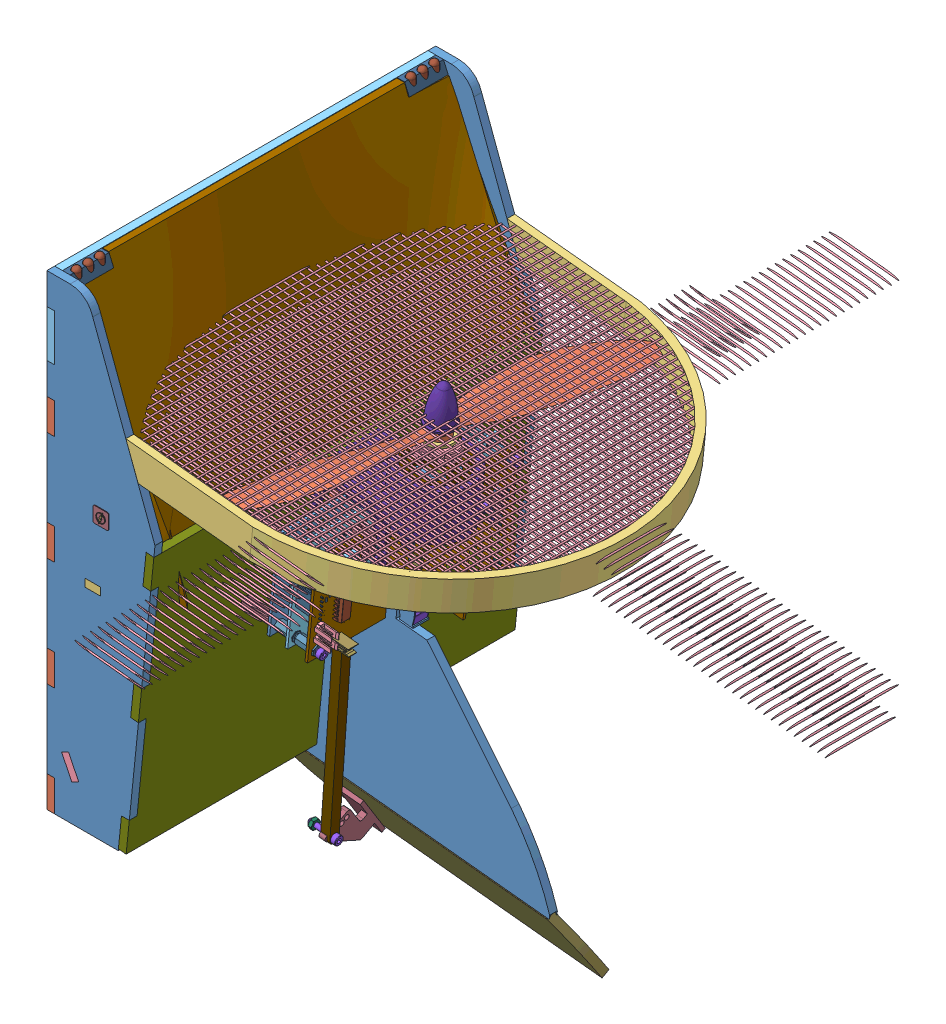
SolidWorks assembly AssTotaleSimu3, configuration Défaut. Lengths in mm. (continued)
Components (placement in the parent): (continued)
- AssStructSimu-1: AssStructSimu [Défaut] at (-125.7658 -1.8483 624.6548) x (1 0 0) z (0 0 -1) size (253.25 324.59 251.6) (continued)
  - AssCarte-1: AssCarte [Défaut] at (38.0121 147.1029 290.772) x (-0.101852 0.9948 0) z (0.9948 0.101852 0) size (66.52 130.57 98.72) (continued)
    - carte_onduleur_v3-1: carte_onduleur_v3 [Défaut] at (-131.8199 12.0892 20.7912) size (66.52 130.57 82.34) (continued)
      - U_DSPIC-1: U_DSPIC [Défaut] at (1.863 -2.61 0.803) size (7.92 35.56 7.75)
        - Open CASCADE STEP translator 6.8 1.17.1-1: Open CASCADE STEP translator 6.8 1.17.1 [Défaut] at origin size (7.92 35.56 7.75)
          - Body_1_4-1: Body_1_4 [Défaut] at (0 -0.2 4) x (1 0 0) z (0 -1 0) size (7.92 7.75 35.56)
      - C_DEC_DSPIC-1: C_DEC_DSPIC [Défaut] at (7.7 -8.8 -0.803) x (0 1 0) z (0 0 -1) size (2.34 1.04 0.5)
        - Open CASCADE STEP translator 6.8 1.6.1-1: Open CASCADE STEP translator 6.8 1.6.1 [Défaut] at origin size (2.34 1.04 0.5)
          - Body_1-1: Body_1 [Défaut] at origin size (2.29 1.04 0.43)
          - Pin_1-1: Pin_1 [Défaut] at (0.3048 0 0) x (-1 0 0) z (0 0 1) size (0.51 1.02 0.5)
          - Pin_2-1: Pin_2 [Défaut] at origin size (0.51 1.02 0.5)
      - IN-1: IN [Défaut] at (24.3 -5.3 0.803) x (0 1 0) z (0 0 1) size (10.21 15.56 26.9)
        - Open CASCADE STEP translator 6.8 1.19.1-1: Open CASCADE STEP translator 6.8 1.19.1 [Défaut] at origin size (10.21 15.56 26.9)
          - Body_1_3-1: Body_1_3 [Défaut] at (-13.5 1.8 3) x (0 1 0) z (1 0 0) size (15.56 26.9 10.21)
            - Imported-1: Imported [Défaut] at (2.0451 -4.5908 20.9802) size (8.6 15.9 10.16)
            - Imported-2: Imported [Défaut] at (-1.6683 9.1092 15.9802) x (0 0 1) z (-1 0 0) size (10.1 18.2 15.1)
              - Imported_2-1: Imported_2 [Défaut] at origin size (10.1 18.2 15.1)
              - Imported_3-1: Imported_3 [Défaut] at origin size (3.43 12.4 4.99)
              - Imported_4-1: Imported_4 [Défaut] at origin size (3.43 12.4 4.99)
              - Imported_5-1: Imported_5 [Défaut] at origin size (3.9 4.9 7)
              - Imported_6-1: Imported_6 [Défaut] at origin size (3.9 4.9 7)
              - Imported_7-1: Imported_7 [Défaut] at origin size (3.8 3.8 6.92)
              - Imported_8-1: Imported_8 [Défaut] at origin size (3.8 3.8 6.92)
              - Imported_9-1: Imported_9 [Défaut] at origin size (9 2.4 14.2)
      - CARTE_CMD-1: CARTE_CMD [Défaut] at (25 57.2 0.803) size (60.1 130 26.62)
        - Open CASCADE STEP translator 6.8 1.20.1-1: Open CASCADE STEP translator 6.8 1.20.1 [Défaut] at origin size (60.1 130 26.62)
          - Body_1_4-1: Body_1_4 [Défaut] at (-55 5 12) size (60.1 130 26.62)
            - 1_2-1: 1_2 [Défaut] at origin size (60.1 130 1.61)
            - 4-1: 4 [Défaut] at (23.6 -124.9 0.803) x (0 1 0) z (0 0 1) size (5 15.24 14.3)
              - =_[0_1_1_4]_2-1: =_[0_1_1_4]_2 [Défaut] at origin size (5 15.24 14.3)
                - 5-1: 5 [Défaut] at (0 -6.5 -13) x (0 1 0) z (0 0 -1) size (15.24 5 14.3)
            - 7-1: 7 [Défaut] at (23.6 -5 0.803) x (0 1 0) z (0 0 1) size (5 15.24 14.3)
              - =_[0_1_1_7]-1: =_[0_1_1_7] [Défaut] at origin size (5 15.24 14.3)
                - 5-1: 5 [Défaut] at (0 -6.5 -13) x (0 1 0) z (0 0 -1) size (15.24 5 14.3)
            - 10_2-1: 10_2 [Défaut] at (18.4 -115.6 0.803) size (25.4 7.92 7.75)
              - =_[0_1_1_9]-1: =_[0_1_1_9] [Défaut] at origin size (25.4 7.92 7.75)
                - 8-1: 8 [Défaut] at (11.2 4 0) x (0 1 0) z (1 0 0) size (7.92 7.75 25.4)
            - 13_2-1: 13_2 [Défaut] at (55.4 -114.7 0.803) x (-1 0 0) z (0 0 1) size (5 7.62 14.3)
              - =_[0_1_1_12]-1: =_[0_1_1_12] [Défaut] at origin size (5 7.62 14.3)
                - 11-1: 11 [Défaut] at (0 -2.5 11) x (0 -1 0) z (0 0 1) size (7.62 5 14.3)
            - 25-1: 25 [Défaut] at (56.9 -12.8 0.803) x (-1 0 0) z (0 0 1) size (16.02 47.26 11.05)
              - =_[0_1_1_15]_2-1: =_[0_1_1_15]_2 [Défaut] at origin size (16.02 47.26 11.05)
                - 23-1: 23 [Défaut] at (-36.5 21 4) x (0 -1 0) z (1 0 0) size (47.26 11.05 16.02)
                  - 14-1: 14 [Défaut] at (-7.4961 -1.5352 42.5833) size (42.58 6.55 16.01)
                  - 22-1: 22 [Défaut] at (19.3039 2.3748 37.905) x (-1 0 0) z (0 0 -1) size (10.36 6.14 15.24)
                    - 21-1: 21 [Défaut] at origin size (10.36 6.14 7.62)
                      - 19_2-1: 19_2 [Défaut] at origin size (10.36 6.14 2.54)
                        - 15-1: 15 [Défaut] at origin size (8.4 2.54 2.54)
                        - 16-1: 16 [Défaut] at (-0.0461 1.2682 1.27) x (0 0 -1) z (0.999998 -0.002105 0) size (1.95 5.07 7.58)
                      - 19_2-2: 19_2 [Défaut] at (0 0 -2.54) size (10.36 6.14 2.54)
                        - 15-1: 15 [Défaut] at origin size (8.4 2.54 2.54)
                        - 16-1: 16 [Défaut] at (-0.0461 1.2682 1.27) x (0 0 -1) z (0.999998 -0.002105 0) size (1.95 5.07 7.58)
                      - 19_2-3: 19_2 [Défaut] at (0 0 -5.08) size (10.36 6.14 2.54)
                        - 15-1: 15 [Défaut] at origin size (8.4 2.54 2.54)
                        - 16-1: 16 [Défaut] at (-0.0461 1.2682 1.27) x (0 0 -1) z (0.999998 -0.002105 0) size (1.95 5.07 7.58)
                    - 21-2: 21 [Défaut] at (0 0 -7.62) size (10.36 6.14 7.62)
                      - 19_2-1: 19_2 [Défaut] at origin size (10.36 6.14 2.54)
                        - 15-1: 15 [Défaut] at origin size (8.4 2.54 2.54)
                        - 16-1: 16 [Défaut] at (-0.0461 1.2682 1.27) x (0 0 -1) z (0.999998 -0.002105 0) size (1.95 5.07 7.58)
                      - 19_2-2: 19_2 [Défaut] at (0 0 -2.54) size (10.36 6.14 2.54)
                        - 15-1: 15 [Défaut] at origin size (8.4 2.54 2.54)
                        - 16-1: 16 [Défaut] at (-0.0461 1.2682 1.27) x (0 0 -1) z (0.999998 -0.002105 0) size (1.95 5.07 7.58)
                      - 19_2-3: 19_2 [Défaut] at (0 0 -5.08) size (10.36 6.14 2.54)
                        - 15-1: 15 [Défaut] at origin size (8.4 2.54 2.54)
                        - 16-1: 16 [Défaut] at (-0.0461 1.2682 1.27) x (0 0 -1) z (0.999998 -0.002105 0) size (1.95 5.07 7.58)
            - 31-1: 31 [Défaut] at (12.9 -104.5 0.803) size (6.76 3.64 4.37)
              - =_[0_1_1_24]-1: =_[0_1_1_24] [Défaut] at origin size (6.76 3.64 4.37)
                - 29-1: 29 [Défaut] at (-0.3 -2 0) size (6.76 3.64 4.37)
                  - =_[0_1_1_3]_3-1: =_[0_1_1_3]_3 [Défaut] at origin size (6 3.64 4.37)
                  - =_[0_1_1_4]_3-1: =_[0_1_1_4]_3 [Défaut] at origin size (0.38 1 0.67)
                  - =_[0_1_1_5]_3-1: =_[0_1_1_5]_3 [Défaut] at origin size (0.38 1 0.67)
            - 36-1: 36 [Défaut] at (28.6 -12.2 0.803) x (0 -1 0) z (0 0 1) size (2.34 1.04 0.5)
              - =_[0_1_1_30]-1: =_[0_1_1_30] [Défaut] at origin size (2.34 1.04 0.5)
                - 32_2-1: 32_2 [Défaut] at origin size (2.29 1.04 0.43)
                - 33_2-1: 33_2 [Défaut] at (0.3048 0 0) x (-1 0 0) z (0 0 1) size (0.51 1.02 0.5)
                - 34-1: 34 [Défaut] at origin size (0.51 1.02 0.5)
            - 38-1: 38 [Défaut] at (23.7 -12.2 0.803) x (0 -1 0) z (0 0 1) size (2.34 1.04 0.5)
              - =_[0_1_1_30]-1: =_[0_1_1_30] [Défaut] at origin size (2.34 1.04 0.5)
                - 32_2-1: 32_2 [Défaut] at origin size (2.29 1.04 0.43)
                - 33_2-1: 33_2 [Défaut] at (0.3048 0 0) x (-1 0 0) z (0 0 1) size (0.51 1.02 0.5)
                - 34-1: 34 [Défaut] at origin size (0.51 1.02 0.5)
            - 40_2-1: 40_2 [Défaut] at (26.2 -12.2 0.803) x (0 -1 0) z (0 0 1) size (2.34 1.04 0.5)
              - =_[0_1_1_30]-1: =_[0_1_1_30] [Défaut] at origin size (2.34 1.04 0.5)
                - 32_2-1: 32_2 [Défaut] at origin size (2.29 1.04 0.43)
                - 33_2-1: 33_2 [Défaut] at (0.3048 0 0) x (-1 0 0) z (0 0 1) size (0.51 1.02 0.5)
                - 34-1: 34 [Défaut] at origin size (0.51 1.02 0.5)
            - 42_2-1: 42_2 [Défaut] at (24.4 -119.2 0.803) size (2.34 1.04 0.5)
              - =_[0_1_1_30]-1: =_[0_1_1_30] [Défaut] at origin size (2.34 1.04 0.5)
                - 32_2-1: 32_2 [Défaut] at origin size (2.29 1.04 0.43)
                - 33_2-1: 33_2 [Défaut] at (0.3048 0 0) x (-1 0 0) z (0 0 1) size (0.51 1.02 0.5)
                - 34-1: 34 [Défaut] at origin size (0.51 1.02 0.5)
            - 45-1: 45 [Défaut] at (46.4 -125 0.803) size (5.08 5 14.3)
              - =_[0_1_1_38]-1: =_[0_1_1_38] [Défaut] at origin size (5.08 5 14.3)
                - 46-1: 46 [Défaut] at (1.2 0 11) size (5.08 5 14.3)
            - 48-1: 48 [Défaut] at (40.1 -125 0.803) size (5.08 5 14.3)
              - =_[0_1_1_41]-1: =_[0_1_1_41] [Défaut] at origin size (5.08 5 14.3)
                - 46-1: 46 [Défaut] at (1.2 0 11) size (5.08 5 14.3)
            - 51-1: 51 [Défaut] at (6.4 -119.9 0.803) x (0 1 0) z (0 0 1) size (15.24 2.54 7.37)
              - =_[0_1_1_43]-1: =_[0_1_1_43] [Défaut] at origin size (15.24 2.54 7.37)
                - 49_2-1: 49_2 [Défaut] at (6.5 0 0) x (1 0 0) z (0 -1 0) size (15.24 7.37 2.54)
            - 57_2-1: 57_2 [Défaut] at (50.8796 -121.1 -0.803) x (-1 0 0) z (0 0 -1) size (2.54 1.98 0.64)
              - =_[0_1_1_46]-1: =_[0_1_1_46] [Défaut] at origin size (2.54 1.98 0.64)
                - 52-1: 52 [Défaut] at origin size (2.54 1.14 0.58)
                - 53-1: 53 [Défaut] x (0 -1 0) z (0 0 1) size (0.43 0.51 0.38)
                - 54-1: 54 [Défaut] at (1.8796 1.8796 0) x (0 -1 0) z (0 0 1) size (0.43 0.51 0.38)
                - 55-1: 55 [Défaut] at (-0.9652 -2.8448 0) x (0 1 0) z (0 0 1) size (0.41 0.51 0.38)
            - 59_2-1: 59_2 [Défaut] at (43.6398 -120.995 -0.803) x (-1 0 0) z (0 0 -1) size (2.54 1.98 0.64)
              - =_[0_1_1_46]-1: =_[0_1_1_46] [Défaut] at origin size (2.54 1.98 0.64)
                - 52-1: 52 [Défaut] at origin size (2.54 1.14 0.58)
                - 53-1: 53 [Défaut] x (0 -1 0) z (0 0 1) size (0.43 0.51 0.38)
                - 54-1: 54 [Défaut] at (1.8796 1.8796 0) x (0 -1 0) z (0 0 1) size (0.43 0.51 0.38)
                - 55-1: 55 [Défaut] at (-0.9652 -2.8448 0) x (0 1 0) z (0 0 1) size (0.41 0.51 0.38)
            - 61_2-1: 61_2 [Défaut] at (47.6 -119.9 -0.803) x (-1 0 0) z (0 0 -1) size (2.34 1.04 0.5)
              - =_[0_1_1_30]-1: =_[0_1_1_30] [Défaut] at origin size (2.34 1.04 0.5)
                - 32_2-1: 32_2 [Défaut] at origin size (2.29 1.04 0.43)
                - 33_2-1: 33_2 [Défaut] at (0.3048 0 0) x (-1 0 0) z (0 0 1) size (0.51 1.02 0.5)
                - 34-1: 34 [Défaut] at origin size (0.51 1.02 0.5)
            - 63-1: 63 [Défaut] at (40.4 -119.9 -0.803) x (-1 0 0) z (0 0 -1) size (2.34 1.04 0.5)
              - =_[0_1_1_30]-1: =_[0_1_1_30] [Défaut] at origin size (2.34 1.04 0.5)
                - 32_2-1: 32_2 [Défaut] at origin size (2.29 1.04 0.43)
                - 33_2-1: 33_2 [Défaut] at (0.3048 0 0) x (-1 0 0) z (0 0 1) size (0.51 1.02 0.5)
                - 34-1: 34 [Défaut] at origin size (0.51 1.02 0.5)
            - 68-1: 68 [Défaut] at (47.7 -21.8 -0.803) x (0 1 0) z (0 0 -1) size (2.34 1.04 0.5)
              - =_[0_1_1_55]-1: =_[0_1_1_55] [Défaut] at origin size (2.34 1.04 0.5)
                - 64-1: 64 [Défaut] at origin size (2.29 1.04 0.43)
                - 65-1: 65 [Défaut] at (0.3048 0 0) x (-1 0 0) z (0 0 1) size (0.51 1.02 0.5)
                - 66-1: 66 [Défaut] at origin size (0.51 1.02 0.5)
            - 70-1: 70 [Défaut] at (47.6 -121.7 -0.803) x (-1 0 0) z (0 0 -1) size (2.34 1.04 0.5)
              - =_[0_1_1_30]-1: =_[0_1_1_30] [Défaut] at origin size (2.34 1.04 0.5)
                - 32_2-1: 32_2 [Défaut] at origin size (2.29 1.04 0.43)
                - 33_2-1: 33_2 [Défaut] at (0.3048 0 0) x (-1 0 0) z (0 0 1) size (0.51 1.02 0.5)
                - 34-1: 34 [Défaut] at origin size (0.51 1.02 0.5)
            - 72_2-1: 72_2 [Défaut] at (40.4 -121.5 -0.803) x (-1 0 0) z (0 0 -1) size (2.34 1.04 0.5)
              - =_[0_1_1_30]-1: =_[0_1_1_30] [Défaut] at origin size (2.34 1.04 0.5)
                - 32_2-1: 32_2 [Défaut] at origin size (2.29 1.04 0.43)
                - 33_2-1: 33_2 [Défaut] at (0.3048 0 0) x (-1 0 0) z (0 0 1) size (0.51 1.02 0.5)
                - 34-1: 34 [Défaut] at origin size (0.51 1.02 0.5)
            - 74_2-1: 74_2 [Défaut] at (47.7 -18.3 -0.803) x (0 1 0) z (0 0 -1) size (2.34 1.04 0.5)
              - =_[0_1_1_55]-1: =_[0_1_1_55] [Défaut] at origin size (2.34 1.04 0.5)
                - 64-1: 64 [Défaut] at origin size (2.29 1.04 0.43)
                - 65-1: 65 [Défaut] at (0.3048 0 0) x (-1 0 0) z (0 0 1) size (0.51 1.02 0.5)
                - 66-1: 66 [Défaut] at origin size (0.51 1.02 0.5)
            - 76_2-1: 76_2 [Défaut] at (45.5 -118.3 -0.803) x (1 0 0) z (0 0 -1) size (2.34 1.04 0.5)
              - =_[0_1_1_30]-1: =_[0_1_1_30] [Défaut] at origin size (2.34 1.04 0.5)
                - 32_2-1: 32_2 [Défaut] at origin size (2.29 1.04 0.43)
                - 33_2-1: 33_2 [Défaut] at (0.3048 0 0) x (-1 0 0) z (0 0 1) size (0.51 1.02 0.5)
                - 34-1: 34 [Défaut] at origin size (0.51 1.02 0.5)
            - 78_2-1: 78_2 [Défaut] at (38.2 -118.3 -0.803) x (1 0 0) z (0 0 -1) size (2.34 1.04 0.5)
              - =_[0_1_1_30]-1: =_[0_1_1_30] [Défaut] at origin size (2.34 1.04 0.5)
                - 32_2-1: 32_2 [Défaut] at origin size (2.29 1.04 0.43)
                - 33_2-1: 33_2 [Défaut] at (0.3048 0 0) x (-1 0 0) z (0 0 1) size (0.51 1.02 0.5)
                - 34-1: 34 [Défaut] at origin size (0.51 1.02 0.5)
            - 80_2-1: 80_2 [Défaut] at (28.6 -10.7 0.803) x (0 1 0) z (0 0 1) size (2.34 1.04 0.5)
              - =_[0_1_1_55]-1: =_[0_1_1_55] [Défaut] at origin size (2.34 1.04 0.5)
                - 64-1: 64 [Défaut] at origin size (2.29 1.04 0.43)
                - 65-1: 65 [Défaut] at (0.3048 0 0) x (-1 0 0) z (0 0 1) size (0.51 1.02 0.5)
                - 66-1: 66 [Défaut] at origin size (0.51 1.02 0.5)
            - 82_2-1: 82_2 [Défaut] at (23.7 -10.7 0.803) x (0 1 0) z (0 0 1) size (2.34 1.04 0.5)
              - =_[0_1_1_55]-1: =_[0_1_1_55] [Défaut] at origin size (2.34 1.04 0.5)
                - 64-1: 64 [Défaut] at origin size (2.29 1.04 0.43)
                - 65-1: 65 [Défaut] at (0.3048 0 0) x (-1 0 0) z (0 0 1) size (0.51 1.02 0.5)
                - 66-1: 66 [Défaut] at origin size (0.51 1.02 0.5)
            - 84-1: 84 [Défaut] at (26.2 -10.7 0.803) x (0 1 0) z (0 0 1) size (2.34 1.04 0.5)
              - =_[0_1_1_55]-1: =_[0_1_1_55] [Défaut] at origin size (2.34 1.04 0.5)
                - 64-1: 64 [Défaut] at origin size (2.29 1.04 0.43)
                - 65-1: 65 [Défaut] at (0.3048 0 0) x (-1 0 0) z (0 0 1) size (0.51 1.02 0.5)
                - 66-1: 66 [Défaut] at origin size (0.51 1.02 0.5)
            - 86-1: 86 [Défaut] at (23.0336 -119.2 0.803) x (-1 0 0) z (0 0 1) size (2.34 1.04 0.5)
              - =_[0_1_1_55]-1: =_[0_1_1_55] [Défaut] at origin size (2.34 1.04 0.5)
                - 64-1: 64 [Défaut] at origin size (2.29 1.04 0.43)
                - 65-1: 65 [Défaut] at (0.3048 0 0) x (-1 0 0) z (0 0 1) size (0.51 1.02 0.5)
                - 66-1: 66 [Défaut] at origin size (0.51 1.02 0.5)
            - 88-1: 88 [Défaut] at (14.1 -114.2 0.803) x (0 -1 0) z (0 0 1) size (2.34 1.04 0.5)
              - =_[0_1_1_55]-1: =_[0_1_1_55] [Défaut] at origin size (2.34 1.04 0.5)
                - 64-1: 64 [Défaut] at origin size (2.29 1.04 0.43)
                - 65-1: 65 [Défaut] at (0.3048 0 0) x (-1 0 0) z (0 0 1) size (0.51 1.02 0.5)
                - 66-1: 66 [Défaut] at origin size (0.51 1.02 0.5)
            - 90-1: 90 [Défaut] at (43.6 -107.8 -0.803) x (1 0 0) z (0 0 -1) size (2.34 1.04 0.5)
              - =_[0_1_1_55]-1: =_[0_1_1_55] [Défaut] at origin size (2.34 1.04 0.5)
                - 64-1: 64 [Défaut] at origin size (2.29 1.04 0.43)
                - 65-1: 65 [Défaut] at (0.3048 0 0) x (-1 0 0) z (0 0 1) size (0.51 1.02 0.5)
                - 66-1: 66 [Défaut] at origin size (0.51 1.02 0.5)
            - 92-1: 92 [Défaut] at (43.6 -106 -0.803) x (1 0 0) z (0 0 -1) size (2.34 1.04 0.5)
              - =_[0_1_1_55]-1: =_[0_1_1_55] [Défaut] at origin size (2.34 1.04 0.5)
                - 64-1: 64 [Défaut] at origin size (2.29 1.04 0.43)
                - 65-1: 65 [Défaut] at (0.3048 0 0) x (-1 0 0) z (0 0 1) size (0.51 1.02 0.5)
                - 66-1: 66 [Défaut] at origin size (0.51 1.02 0.5)
            - 175-1: 175 [Défaut] at (10 -21.7 0.803) x (0 -1 0) z (0 0 1) size (18.3 25.4 12.7)
              - =_[0_1_1_72]-1: =_[0_1_1_72] [Défaut] at origin size (18.3 25.4 12.7)
                - 173-1: 173 [Défaut] at (-1.4 -1 12) x (-1 0 0) z (0 1 0) size (18.3 12.7 25.4)
                  - board_1-1: board_1 [Défaut] at (-7.5 -1.57 12.5) size (15 1.57 25)
                  - hole_plating_20-1: hole_plating_20 [Défaut] at (-1.5 0 23.93) size (1.5 0.01 1.5)
                  - hole_plating_20-2: hole_plating_20 [Défaut] at (-1.5 0 21.39) size (1.5 0.01 1.5)
                  - hole_plating_20-3: hole_plating_20 [Défaut] at (-1.5 0 8.69) size (1.5 0.01 1.5)
                  - hole_plating_20-4: hole_plating_20 [Défaut] at (-1.5 -1.58 13.77) size (1.5 0.01 1.5)
                  - hole_plating_20-5: hole_plating_20 [Défaut] at (-1.5 0 16.31) size (1.5 0.01 1.5)
                  - hole_plating_20-6: hole_plating_20 [Défaut] at (-1.5 0 18.85) size (1.5 0.01 1.5)
                  - hole_plating_20-7: hole_plating_20 [Défaut] at (-1.5 0 13.77) size (1.5 0.01 1.5)
                  - hole_plating_20-8: hole_plating_20 [Défaut] at (-1.5 -1.58 11.23) size (1.5 0.01 1.5)
                  - hole_plating_20-9: hole_plating_20 [Défaut] at (-1.5 -1.58 18.85) size (1.5 0.01 1.5)
                  - hole_plating_20-10: hole_plating_20 [Défaut] at (-1.5 -1.58 6.15) size (1.5 0.01 1.5)
                  - hole_plating_20-11: hole_plating_20 [Défaut] at (-1.5 0 1.07) size (1.5 0.01 1.5)
                  - hole_plating_20-12: hole_plating_20 [Défaut] at (-1.5 -1.58 3.61) size (1.5 0.01 1.5)
                  - hole_plating_20-13: hole_plating_20 [Défaut] at (-1.5 -1.58 1.07) size (1.5 0.01 1.5)
                  - hole_plating_20-14: hole_plating_20 [Défaut] at (-1.5 -1.58 8.69) size (1.5 0.01 1.5)
                  - hole_plating_20-15: hole_plating_20 [Défaut] at (-1.5 -1.58 16.31) size (1.5 0.01 1.5)
                  - hole_plating_20-16: hole_plating_20 [Défaut] at (-1.5 0 11.23) size (1.5 0.01 1.5)
                  - hole_plating_20-17: hole_plating_20 [Défaut] at (-1.5 0 3.61) size (1.5 0.01 1.5)
                  - hole_plating_20-18: hole_plating_20 [Défaut] at (-1.5 -1.58 21.39) size (1.5 0.01 1.5)
                  - hole_plating_20-19: hole_plating_20 [Défaut] at (-1.5 0 6.15) size (1.5 0.01 1.5)
                  - hole_plating_20-20: hole_plating_20 [Défaut] at (-1.5 -1.58 23.93) size (1.5 0.01 1.5)
                  - Pin_Header_1x10_TH_Pitch_2.54mm_1-1: Pin_Header_1x10_TH_Pitch_2.54mm_1 [Défaut] at (-1.5 -1.5786 23.93) x (0 0 -1) z (0 -1 0) size (25.4 2.54 12.7)
                    - 124-1: 124 [Défaut] at origin size (25.4 2.54 2.8)
                      - =_[0_1_1_77]-1: =_[0_1_1_77] [Défaut] at origin size (2.54 2.54 2.8)
                      - =_[0_1_1_79]-1: =_[0_1_1_79] [Défaut] at origin size (2.54 2.54 2.8)
                      - =_[0_1_1_80]-1: =_[0_1_1_80] [Défaut] at origin size (2.54 2.54 2.8)
                      - =_[0_1_1_81]-1: =_[0_1_1_81] [Défaut] at origin size (2.54 2.54 2.8)
                      - =_[0_1_1_82]-1: =_[0_1_1_82] [Défaut] at origin size (2.54 2.54 2.8)
                      - =_[0_1_1_83]-1: =_[0_1_1_83] [Défaut] at origin size (2.54 2.54 2.8)
                      - =_[0_1_1_84]-1: =_[0_1_1_84] [Défaut] at origin size (2.54 2.54 2.8)
                      - =_[0_1_1_85]-1: =_[0_1_1_85] [Défaut] at origin size (2.54 2.54 2.8)
                      - =_[0_1_1_86]-1: =_[0_1_1_86] [Défaut] at origin size (2.54 2.54 2.8)
                      - =_[0_1_1_87]-1: =_[0_1_1_87] [Défaut] at origin size (2.54 2.54 2.8)
                    - 135-1: 135 [Défaut] at origin size (23.49 0.63 12.7)
                      - =_[0_1_1_88]-1: =_[0_1_1_88] [Défaut] at origin size (0.63 0.63 12.7)
                      - =_[0_1_1_90]-1: =_[0_1_1_90] [Défaut] at origin size (0.63 0.63 12.7)
                      - =_[0_1_1_91]-1: =_[0_1_1_91] [Défaut] at origin size (0.63 0.63 12.7)
                      - =_[0_1_1_92]-1: =_[0_1_1_92] [Défaut] at origin size (0.63 0.63 12.7)
                      - =_[0_1_1_93]-1: =_[0_1_1_93] [Défaut] at origin size (0.63 0.63 12.7)
                      - =_[0_1_1_94]-1: =_[0_1_1_94] [Défaut] at origin size (0.63 0.63 12.7)
                      - =_[0_1_1_95]-1: =_[0_1_1_95] [Défaut] at origin size (0.63 0.63 12.7)
                      - =_[0_1_1_96]-1: =_[0_1_1_96] [Défaut] at origin size (0.63 0.63 12.7)
                      - =_[0_1_1_97]-1: =_[0_1_1_97] [Défaut] at origin size (0.63 0.63 12.7)
                      - =_[0_1_1_98]-1: =_[0_1_1_98] [Défaut] at origin size (0.63 0.63 12.7)
                  - MPU-9250_1-1: MPU-9250_1 [Défaut] at (-8 0.05 12.5) x (-1 0 0) z (0 1 0) size (3 3 1.05)
                  - tantalum_10uF_1-1: tantalum_10uF_1 [Défaut] at (-13.167 0.1 10.9372) x (0 0 1) z (0 1 0) size (3.4 1.6 1.71)
                  - SOT23_5_1-1: SOT23_5_1 [Défaut] at (-7.475 -0.0136 21) x (0 0 1) z (0 1 0) size (3 3.2 0.92)
                  - RESC-0603_5-1: RESC-0603_5 [Défaut] at (-6.85 0 7.45) x (1 0 0) z (0 1 0) size (1.7 0.9 0.55)
                    - 143-1: 143 [Défaut] at origin size (1.7 0.9 0.55)
                      - =_[0_1_1_103]-1: =_[0_1_1_103] [Défaut] at origin size (0.4 0.9 0.53)
                      - =_[0_1_1_105]-1: =_[0_1_1_105] [Défaut] at origin size (0.4 0.9 0.53)
                      - =_[0_1_1_106]-1: =_[0_1_1_106] [Défaut] at origin size (1.64 0.9 0.52)
                    - 152-1: 152 [Défaut] at origin
                      - =_[0_1_1_107]-1: =_[0_1_1_107] [Défaut] at origin
                      - =_[0_1_1_109]-1: =_[0_1_1_109] [Défaut] at origin
                      - =_[0_1_1_110]-1: =_[0_1_1_110] [Défaut] at origin
                      - =_[0_1_1_111]-1: =_[0_1_1_111] [Défaut] at origin
                      - =_[0_1_1_112]-1: =_[0_1_1_112] [Défaut] at origin
                      - =_[0_1_1_113]-1: =_[0_1_1_113] [Défaut] at origin
                      - =_[0_1_1_114]-1: =_[0_1_1_114] [Défaut] at origin
                      - =_[0_1_1_115]-1: =_[0_1_1_115] [Défaut] at origin
                  - RESC-0603_5-2: RESC-0603_5 [Défaut] at (-9.85 0 16.05) x (1 0 0) z (0 1 0) size (1.7 0.9 0.55)
                    - 143-1: 143 [Défaut] at origin size (1.7 0.9 0.55)
                      - =_[0_1_1_103]-1: =_[0_1_1_103] [Défaut] at origin size (0.4 0.9 0.53)
                      - =_[0_1_1_105]-1: =_[0_1_1_105] [Défaut] at origin size (0.4 0.9 0.53)
                      - =_[0_1_1_106]-1: =_[0_1_1_106] [Défaut] at origin size (1.64 0.9 0.52)
                    - 152-1: 152 [Défaut] at origin
                      - =_[0_1_1_107]-1: =_[0_1_1_107] [Défaut] at origin
                      - =_[0_1_1_109]-1: =_[0_1_1_109] [Défaut] at origin
                      - =_[0_1_1_110]-1: =_[0_1_1_110] [Défaut] at origin
                      - =_[0_1_1_111]-1: =_[0_1_1_111] [Défaut] at origin
                      - =_[0_1_1_112]-1: =_[0_1_1_112] [Défaut] at origin
                      - =_[0_1_1_113]-1: =_[0_1_1_113] [Défaut] at origin
                      - =_[0_1_1_114]-1: =_[0_1_1_114] [Défaut] at origin
                      - =_[0_1_1_115]-1: =_[0_1_1_115] [Défaut] at origin
                  - RESC-0603_5-3: RESC-0603_5 [Défaut] at (-6.85 0 17.55) x (1 0 0) z (0 1 0) size (1.7 0.9 0.55)
                    - 143-1: 143 [Défaut] at origin size (1.7 0.9 0.55)
                      - =_[0_1_1_103]-1: =_[0_1_1_103] [Défaut] at origin size (0.4 0.9 0.53)
                      - =_[0_1_1_105]-1: =_[0_1_1_105] [Défaut] at origin size (0.4 0.9 0.53)
                      - =_[0_1_1_106]-1: =_[0_1_1_106] [Défaut] at origin size (1.64 0.9 0.52)
                    - 152-1: 152 [Défaut] at origin
                      - =_[0_1_1_107]-1: =_[0_1_1_107] [Défaut] at origin
                      - =_[0_1_1_109]-1: =_[0_1_1_109] [Défaut] at origin
                      - =_[0_1_1_110]-1: =_[0_1_1_110] [Défaut] at origin
                      - =_[0_1_1_111]-1: =_[0_1_1_111] [Défaut] at origin
                      - =_[0_1_1_112]-1: =_[0_1_1_112] [Défaut] at origin
                      - =_[0_1_1_113]-1: =_[0_1_1_113] [Défaut] at origin
                      - =_[0_1_1_114]-1: =_[0_1_1_114] [Défaut] at origin
                      - =_[0_1_1_115]-1: =_[0_1_1_115] [Défaut] at origin
                  - RESC-0603_5-4: RESC-0603_5 [Défaut] at (-6.85 0 16.05) x (1 0 0) z (0 1 0) size (1.7 0.9 0.55)
                    - 143-1: 143 [Défaut] at origin size (1.7 0.9 0.55)
                      - =_[0_1_1_103]-1: =_[0_1_1_103] [Défaut] at origin size (0.4 0.9 0.53)
                      - =_[0_1_1_105]-1: =_[0_1_1_105] [Défaut] at origin size (0.4 0.9 0.53)
                      - =_[0_1_1_106]-1: =_[0_1_1_106] [Défaut] at origin size (1.64 0.9 0.52)
                    - 152-1: 152 [Défaut] at origin
                      - =_[0_1_1_107]-1: =_[0_1_1_107] [Défaut] at origin
                      - =_[0_1_1_109]-1: =_[0_1_1_109] [Défaut] at origin
                      - =_[0_1_1_110]-1: =_[0_1_1_110] [Défaut] at origin
                      - =_[0_1_1_111]-1: =_[0_1_1_111] [Défaut] at origin
                      - =_[0_1_1_112]-1: =_[0_1_1_112] [Défaut] at origin
                      - =_[0_1_1_113]-1: =_[0_1_1_113] [Défaut] at origin
                      - =_[0_1_1_114]-1: =_[0_1_1_114] [Défaut] at origin
                      - =_[0_1_1_115]-1: =_[0_1_1_115] [Défaut] at origin
                  - RESC-0603_5-5: RESC-0603_5 [Défaut] at (-6.85 0 5.95) x (1 0 0) z (0 1 0) size (1.7 0.9 0.55)
                    - 143-1: 143 [Défaut] at origin size (1.7 0.9 0.55)
                      - =_[0_1_1_103]-1: =_[0_1_1_103] [Défaut] at origin size (0.4 0.9 0.53)
                      - =_[0_1_1_105]-1: =_[0_1_1_105] [Défaut] at origin size (0.4 0.9 0.53)
                      - =_[0_1_1_106]-1: =_[0_1_1_106] [Défaut] at origin size (1.64 0.9 0.52)
                    - 152-1: 152 [Défaut] at origin
                      - =_[0_1_1_107]-1: =_[0_1_1_107] [Défaut] at origin
                      - =_[0_1_1_109]-1: =_[0_1_1_109] [Défaut] at origin
                      - =_[0_1_1_110]-1: =_[0_1_1_110] [Défaut] at origin
                      - =_[0_1_1_111]-1: =_[0_1_1_111] [Défaut] at origin
                      - =_[0_1_1_112]-1: =_[0_1_1_112] [Défaut] at origin
                      - =_[0_1_1_113]-1: =_[0_1_1_113] [Défaut] at origin
                      - =_[0_1_1_114]-1: =_[0_1_1_114] [Défaut] at origin
                      - =_[0_1_1_115]-1: =_[0_1_1_115] [Défaut] at origin
                  - CAPC-0603-T0.9-BN_5-1: CAPC-0603-T0.9-BN_5 [Défaut] at (-9.85 0 8.95) x (1 0 0) z (0 1 0) size (1.7 0.9 0.9)
                    - =_[0_1_1_117]-1: =_[0_1_1_117] [Défaut] at origin size (1.7 0.9 0.9)
                    - 167-1: 167 [Défaut] at origin
                      - =_[0_1_1_118]-1: =_[0_1_1_118] [Défaut] at origin
                      - =_[0_1_1_120]-1: =_[0_1_1_120] [Défaut] at origin
                      - =_[0_1_1_121]-1: =_[0_1_1_121] [Défaut] at origin
                      - =_[0_1_1_122]-1: =_[0_1_1_122] [Défaut] at origin
                      - =_[0_1_1_123]-1: =_[0_1_1_123] [Défaut] at origin
                      - =_[0_1_1_124]-1: =_[0_1_1_124] [Défaut] at origin
                      - =_[0_1_1_125]-1: =_[0_1_1_125] [Défaut] at origin
                      - =_[0_1_1_126]-1: =_[0_1_1_126] [Défaut] at origin
                  - CAPC-0603-T0.9-BN_5-2: CAPC-0603-T0.9-BN_5 [Défaut] at (-6.85 0 8.95) x (1 0 0) z (0 1 0) size (1.7 0.9 0.9)
                    - =_[0_1_1_117]-1: =_[0_1_1_117] [Défaut] at origin size (1.7 0.9 0.9)
                    - 167-1: 167 [Défaut] at origin
                      - =_[0_1_1_118]-1: =_[0_1_1_118] [Défaut] at origin
                      - =_[0_1_1_120]-1: =_[0_1_1_120] [Défaut] at origin
                      - =_[0_1_1_121]-1: =_[0_1_1_121] [Défaut] at origin
                      - =_[0_1_1_122]-1: =_[0_1_1_122] [Défaut] at origin
                      - =_[0_1_1_123]-1: =_[0_1_1_123] [Défaut] at origin
                      - =_[0_1_1_124]-1: =_[0_1_1_124] [Défaut] at origin
                      - =_[0_1_1_125]-1: =_[0_1_1_125] [Défaut] at origin
                      - =_[0_1_1_126]-1: =_[0_1_1_126] [Défaut] at origin
                  - CAPC-0603-T0.9-BN_5-3: CAPC-0603-T0.9-BN_5 [Défaut] at (-6.85 0 19.05) x (1 0 0) z (0 1 0) size (1.7 0.9 0.9)
                    - =_[0_1_1_117]-1: =_[0_1_1_117] [Défaut] at origin size (1.7 0.9 0.9)
                    - 167-1: 167 [Défaut] at origin
                      - =_[0_1_1_118]-1: =_[0_1_1_118] [Défaut] at origin
                      - =_[0_1_1_120]-1: =_[0_1_1_120] [Défaut] at origin
                      - =_[0_1_1_121]-1: =_[0_1_1_121] [Défaut] at origin
                      - =_[0_1_1_122]-1: =_[0_1_1_122] [Défaut] at origin
                      - =_[0_1_1_123]-1: =_[0_1_1_123] [Défaut] at origin
                      - =_[0_1_1_124]-1: =_[0_1_1_124] [Défaut] at origin
                      - =_[0_1_1_125]-1: =_[0_1_1_125] [Défaut] at origin
                      - =_[0_1_1_126]-1: =_[0_1_1_126] [Défaut] at origin
                  - CAPC-0603-T0.9-BN_5-4: CAPC-0603-T0.9-BN_5 [Défaut] at (-9.85 0 7.45) x (1 0 0) z (0 1 0) size (1.7 0.9 0.9)
                    - =_[0_1_1_117]-1: =_[0_1_1_117] [Défaut] at origin size (1.7 0.9 0.9)
                    - 167-1: 167 [Défaut] at origin
                      - =_[0_1_1_118]-1: =_[0_1_1_118] [Défaut] at origin
                      - =_[0_1_1_120]-1: =_[0_1_1_120] [Défaut] at origin
                      - =_[0_1_1_121]-1: =_[0_1_1_121] [Défaut] at origin
                      - =_[0_1_1_122]-1: =_[0_1_1_122] [Défaut] at origin
                      - =_[0_1_1_123]-1: =_[0_1_1_123] [Défaut] at origin
                      - =_[0_1_1_124]-1: =_[0_1_1_124] [Défaut] at origin
                      - =_[0_1_1_125]-1: =_[0_1_1_125] [Défaut] at origin
                      - =_[0_1_1_126]-1: =_[0_1_1_126] [Défaut] at origin
                  - CAPC-0603-T0.9-BN_5-5: CAPC-0603-T0.9-BN_5 [Défaut] at (-9.85 0 17.55) x (1 0 0) z (0 1 0) size (1.7 0.9 0.9)
                    - =_[0_1_1_117]-1: =_[0_1_1_117] [Défaut] at origin size (1.7 0.9 0.9)
                    - 167-1: 167 [Défaut] at origin
                      - =_[0_1_1_118]-1: =_[0_1_1_118] [Défaut] at origin
                      - =_[0_1_1_120]-1: =_[0_1_1_120] [Défaut] at origin
                      - =_[0_1_1_121]-1: =_[0_1_1_121] [Défaut] at origin
                      - =_[0_1_1_122]-1: =_[0_1_1_122] [Défaut] at origin
                      - =_[0_1_1_123]-1: =_[0_1_1_123] [Défaut] at origin
                      - =_[0_1_1_124]-1: =_[0_1_1_124] [Défaut] at origin
                      - =_[0_1_1_125]-1: =_[0_1_1_125] [Défaut] at origin
                      - =_[0_1_1_126]-1: =_[0_1_1_126] [Défaut] at origin
            - 177-1: 177 [Défaut] at (52.1 -16.5 -0.803) x (1 0 0) z (0 0 -1) size (2.34 1.04 0.5)
              - =_[0_1_1_30]-1: =_[0_1_1_30] [Défaut] at origin size (2.34 1.04 0.5)
                - 32_2-1: 32_2 [Défaut] at origin size (2.29 1.04 0.43)
                - 33_2-1: 33_2 [Défaut] at (0.3048 0 0) x (-1 0 0) z (0 0 1) size (0.51 1.02 0.5)
                - 34-1: 34 [Défaut] at origin size (0.51 1.02 0.5)
            - 179-1: 179 [Défaut] at (22.5336 -121.5 -0.803) x (-1 0 0) z (0 0 -1) size (2.34 1.04 0.5)
              - =_[0_1_1_30]-1: =_[0_1_1_30] [Défaut] at origin size (2.34 1.04 0.5)
                - 32_2-1: 32_2 [Défaut] at origin size (2.29 1.04 0.43)
                - 33_2-1: 33_2 [Défaut] at (0.3048 0 0) x (-1 0 0) z (0 0 1) size (0.51 1.02 0.5)
                - 34-1: 34 [Défaut] at origin size (0.51 1.02 0.5)
            - 181-1: 181 [Défaut] at (48.6 -127 -0.803) x (-1 0 0) z (0 0 -1) size (2.34 1.04 0.5)
              - =_[0_1_1_30]-1: =_[0_1_1_30] [Défaut] at origin size (2.34 1.04 0.5)
                - 32_2-1: 32_2 [Défaut] at origin size (2.29 1.04 0.43)
                - 33_2-1: 33_2 [Défaut] at (0.3048 0 0) x (-1 0 0) z (0 0 1) size (0.51 1.02 0.5)
                - 34-1: 34 [Défaut] at origin size (0.51 1.02 0.5)
            - 183-1: 183 [Défaut] at (26.0189 -121.5 0.803) size (2.34 1.04 0.5)
              - =_[0_1_1_30]-1: =_[0_1_1_30] [Défaut] at origin size (2.34 1.04 0.5)
                - 32_2-1: 32_2 [Défaut] at origin size (2.29 1.04 0.43)
                - 33_2-1: 33_2 [Défaut] at (0.3048 0 0) x (-1 0 0) z (0 0 1) size (0.51 1.02 0.5)
                - 34-1: 34 [Défaut] at origin size (0.51 1.02 0.5)
            - 185-1: 185 [Défaut] at (30.3664 -19 -0.803) x (1 0 0) z (0 0 -1) size (2.34 1.04 0.5)
              - =_[0_1_1_30]-1: =_[0_1_1_30] [Défaut] at origin size (2.34 1.04 0.5)
                - 32_2-1: 32_2 [Défaut] at origin size (2.29 1.04 0.43)
                - 33_2-1: 33_2 [Défaut] at (0.3048 0 0) x (-1 0 0) z (0 0 1) size (0.51 1.02 0.5)
                - 34-1: 34 [Défaut] at origin size (0.51 1.02 0.5)
            - 187-1: 187 [Défaut] at (51.7 -114.3 -0.803) x (0 1 0) z (0 0 -1) size (2.34 1.04 0.5)
              - =_[0_1_1_30]-1: =_[0_1_1_30] [Défaut] at origin size (2.34 1.04 0.5)
                - 32_2-1: 32_2 [Défaut] at origin size (2.29 1.04 0.43)
                - 33_2-1: 33_2 [Défaut] at (0.3048 0 0) x (-1 0 0) z (0 0 1) size (0.51 1.02 0.5)
                - 34-1: 34 [Défaut] at origin size (0.51 1.02 0.5)
            - 189-1: 189 [Défaut] at (50 -114.3 -0.803) x (0 1 0) z (0 0 -1) size (2.34 1.04 0.5)
              - =_[0_1_1_30]-1: =_[0_1_1_30] [Défaut] at origin size (2.34 1.04 0.5)
                - 32_2-1: 32_2 [Défaut] at origin size (2.29 1.04 0.43)
                - 33_2-1: 33_2 [Défaut] at (0.3048 0 0) x (-1 0 0) z (0 0 1) size (0.51 1.02 0.5)
                - 34-1: 34 [Défaut] at origin size (0.51 1.02 0.5)
      - C2_1-1: C2_1 [Défaut] at (-20.6984 1.8 -0.803) x (1 0 0) z (0 0 -1) size (2.34 1.04 0.5)
        - Open CASCADE STEP translator 6.8 1.6.1-1: Open CASCADE STEP translator 6.8 1.6.1 [Défaut] at origin size (2.34 1.04 0.5)
          - Body_1-1: Body_1 [Défaut] at origin size (2.29 1.04 0.43)
          - Pin_1-1: Pin_1 [Défaut] at (0.3048 0 0) x (-1 0 0) z (0 0 1) size (0.51 1.02 0.5)
          - Pin_2-1: Pin_2 [Défaut] at origin size (0.51 1.02 0.5)
      - C2_2-1: C2_2 [Défaut] at (-24.2 1.8 -0.803) x (1 0 0) z (0 0 -1) size (2.34 1.04 0.5)
        - Open CASCADE STEP translator 6.8 1.6.1-1: Open CASCADE STEP translator 6.8 1.6.1 [Défaut] at origin size (2.34 1.04 0.5)
          - Body_1-1: Body_1 [Défaut] at origin size (2.29 1.04 0.43)
          - Pin_1-1: Pin_1 [Défaut] at (0.3048 0 0) x (-1 0 0) z (0 0 1) size (0.51 1.02 0.5)
          - Pin_2-1: Pin_2 [Défaut] at origin size (0.51 1.02 0.5)
      - C3_1-1: C3_1 [Défaut] at (-20.9176 -12.8 -0.803) x (1 0 0) z (0 0 -1) size (2.34 1.04 0.5)
        - Open CASCADE STEP translator 6.8 1.6.1-1: Open CASCADE STEP translator 6.8 1.6.1 [Défaut] at origin size (2.34 1.04 0.5)
          - Body_1-1: Body_1 [Défaut] at origin size (2.29 1.04 0.43)
          - Pin_1-1: Pin_1 [Défaut] at (0.3048 0 0) x (-1 0 0) z (0 0 1) size (0.51 1.02 0.5)
          - Pin_2-1: Pin_2 [Défaut] at origin size (0.51 1.02 0.5)
      - C3_2-1: C3_2 [Défaut] at (-24.4 -12.8 -0.803) x (1 0 0) z (0 0 -1) size (2.34 1.04 0.5)
        - Open CASCADE STEP translator 6.8 1.6.1-1: Open CASCADE STEP translator 6.8 1.6.1 [Défaut] at origin size (2.34 1.04 0.5)
          - Body_1-1: Body_1 [Défaut] at origin size (2.29 1.04 0.43)
          - Pin_1-1: Pin_1 [Défaut] at (0.3048 0 0) x (-1 0 0) z (0 0 1) size (0.51 1.02 0.5)
          - Pin_2-1: Pin_2 [Défaut] at origin size (0.51 1.02 0.5)
      - D_CUR-1: D_CUR [Défaut] at (-12.4432 3.85 -0.803) x (0 -1 0) z (0 0 -1) size (2.7 5.2 1.11)
        - Open CASCADE STEP translator 6.8 1.25.1-1: Open CASCADE STEP translator 6.8 1.25.1 [Défaut] at origin size (2.7 5.2 1.11)
          - Body_1_5-1: Body_1_5 [Défaut] at (1.2 -4 0) x (0 1 0) z (0 0 1) size (5.2 2.7 1.11)
            - =_[0_1_1_3]_4-1: =_[0_1_1_3]_4 [Défaut] at origin size (0.39 0.64 0.01)
            - =_[0_1_1_4]_4-1: =_[0_1_1_4]_4 [Défaut] at origin size (0.6 1.9 0.2)
            - =_[0_1_1_5]_4-1: =_[0_1_1_5]_4 [Défaut] at origin size (0.21 0.08 0.01)
            - =_[0_1_1_6]_2-1: =_[0_1_1_6]_2 [Défaut] at origin size (0.6 1.9 0.2)
            - =_[0_1_1_7]_2-1: =_[0_1_1_7]_2 [Défaut] at origin size (0.46 0.68 0.01)
            - =_[0_1_1_8]_2-1: =_[0_1_1_8]_2 [Défaut] at origin size (0.38 0.66 0.01)
            - =_[0_1_1_9]-1: =_[0_1_1_9] [Défaut] at origin size (0.2 0.62 0.01)
            - =_[0_1_1_10]-1: =_[0_1_1_10] [Défaut] at origin size (4 2.7 1.1)
            - =_[0_1_1_11]-1: =_[0_1_1_11] [Défaut] at origin size (0.46 0.63 0.01)
            - =_[0_1_1_12]-1: =_[0_1_1_12] [Défaut] at origin size (0.56 0.68 0.01)
      - RC1_1-1: RC1_1 [Défaut] at (-20.7176 8.1 -0.803) x (1 0 0) z (0 0 -1) size (2.34 1.04 0.5)
        - Open CASCADE STEP translator 6.8 1.12.1-1: Open CASCADE STEP translator 6.8 1.12.1 [Défaut] at origin size (2.34 1.04 0.5)
          - Body_1_3-1: Body_1_3 [Défaut] at origin size (2.29 1.04 0.43)
          - Pin_1_2-1: Pin_1_2 [Défaut] at (0.3048 0 0) x (-1 0 0) z (0 0 1) size (0.51 1.02 0.5)
          - Pin_2_2-1: Pin_2_2 [Défaut] at origin size (0.51 1.02 0.5)
      - RC1_2-1: RC1_2 [Défaut] at (-22 8.1 -0.803) x (-1 0 0) z (0 0 -1) size (2.34 1.04 0.5)
        - Open CASCADE STEP translator 6.8 1.12.1-1: Open CASCADE STEP translator 6.8 1.12.1 [Défaut] at origin size (2.34 1.04 0.5)
          - Body_1_3-1: Body_1_3 [Défaut] at origin size (2.29 1.04 0.43)
          - Pin_1_2-1: Pin_1_2 [Défaut] at (0.3048 0 0) x (-1 0 0) z (0 0 1) size (0.51 1.02 0.5)
          - Pin_2_2-1: Pin_2_2 [Défaut] at origin size (0.51 1.02 0.5)
      - RC2_1-1: RC2_1 [Défaut] at (-20.716 0.243 -0.803) x (1 0 0) z (0 0 -1) size (2.34 1.04 0.5)
        - Open CASCADE STEP translator 6.8 1.12.1-1: Open CASCADE STEP translator 6.8 1.12.1 [Défaut] at origin size (2.34 1.04 0.5)
          - Body_1_3-1: Body_1_3 [Défaut] at origin size (2.29 1.04 0.43)
          - Pin_1_2-1: Pin_1_2 [Défaut] at (0.3048 0 0) x (-1 0 0) z (0 0 1) size (0.51 1.02 0.5)
          - Pin_2_2-1: Pin_2_2 [Défaut] at origin size (0.51 1.02 0.5)
      - RC2_2-1: RC2_2 [Défaut] at (-22 0.18 -0.803) x (-1 0 0) z (0 0 -1) size (2.34 1.04 0.5)
        - Open CASCADE STEP translator 6.8 1.12.1-1: Open CASCADE STEP translator 6.8 1.12.1 [Défaut] at origin size (2.34 1.04 0.5)
          - Body_1_3-1: Body_1_3 [Défaut] at origin size (2.29 1.04 0.43)
          - Pin_1_2-1: Pin_1_2 [Défaut] at (0.3048 0 0) x (-1 0 0) z (0 0 1) size (0.51 1.02 0.5)
